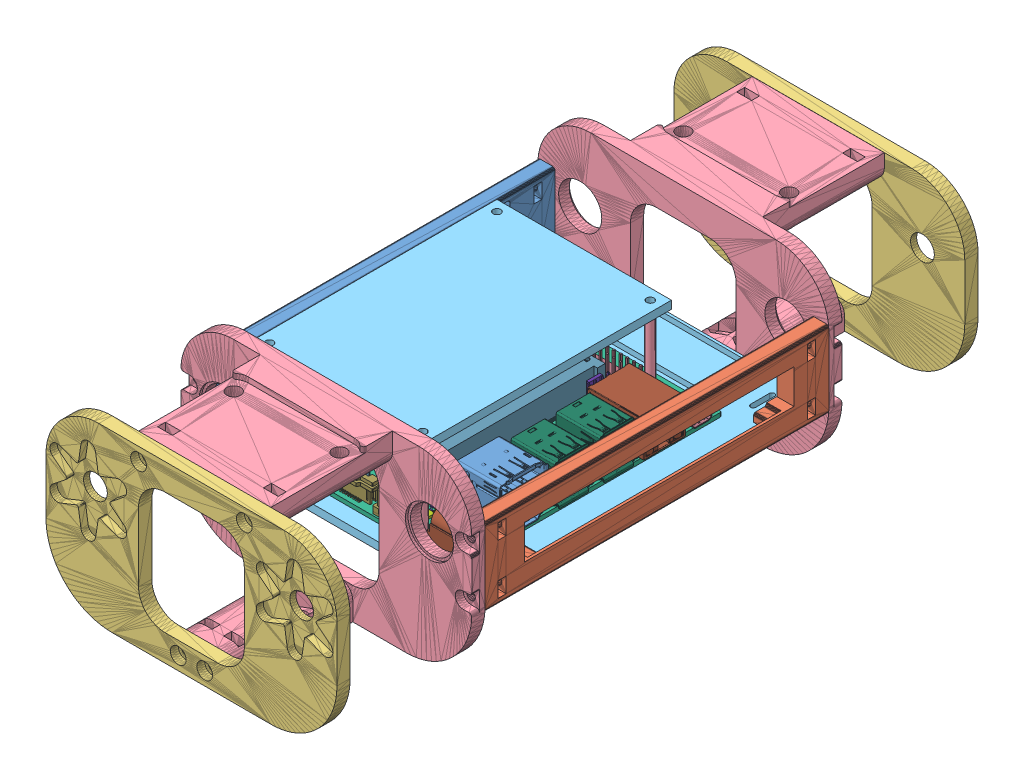
SolidWorks assembly torsol_with_jestson, configuration Default. Lengths in mm.
Overall size (110.41 70.14 242.41).
415 component instances, 78 part files, 32 mates.
Components (placement in the parent):
- R_side_plate-1: R_side_plate [Default] at (-145.3547 -0.5404 -42.0354) x (1 0 0) z (0 -1 0) size (6.5 130 29)
- non-mega_L_side_plate_jetson-2: non-mega_L_side_plate_jetson [Default] at (-41.8547 39.5958 -42.0354) x (-1 0 0) z (0 1 0) size (6.5 130 29)
- O_shoulder-1: O_shoulder [Default] at (-38.1905 81.6503 -93.0354) x (-1 0 0) z (0 -1 0) size (110 5.21 66)
- I_shoulder_mg-1: I_shoulder_mg [Default] at (-38.6047 81.5958 -42.0354) x (-1 0 0) z (0 -1 0) size (110 51 70)
- I_shoulder_mg-2: I_shoulder_mg [Default] at (-148.6047 81.4596 87.9646) x (1 0 0) z (0 -1 0) size (110 51 70)
- O_shoulder-2: O_shoulder [Default] at (-148.6047 81.4596 138.9646) x (1 0 0) z (0 -1 0) size (110 5.21 66)
- plate_with_jetson-1: plate_with_jetson [Default] at (-139.2728 38.0458 18.6623) x (-1 0 0) z (0 -1 0) size (107 134 44.9)
  - plate_jetson-1: plate_jetson [Default] at (-46.1681 -3.8023 -1.45) size (107 130 2.9)
  - Jetson nano_fixed.step-1: Jetson nano_fixed.step [Default] at (-69.1681 -61.3023 -1.45) x (0 1 0) z (0 0 -1) size (100 81.03 30.51)
    - 142-13449-1000-A02_ASM.step-1: 142-13449-1000-A02_ASM.step [Default] at origin size (100 81.03 23.19)
      - 142-13449-1000-A02.step-1: 142-13449-1000-A02.step [Default] at origin size (100 79 1.57)
      - 315-1109-000_1.step-1: 315-1109-000_1.step [Default] at (5.6 4.9 1.575) x (-1 0 0) z (0 0 1) size (4.5 3.5 0.8)
      - 0402_H040.step-1: 0402_H040.step [Default] at (8 -0.825 1.575) size (1 0.5 0.4)
      - 0402_H060.step-1: 0402_H060.step [Default] at (1 5 1.575) x (0 -1 0) z (0 0 1) size (1 0.5 0.6)
      - 0402_H040.step-2: 0402_H040.step [Default] at (9.9 -0.3 1.575) size (1 0.5 0.4)
      - 0402_H040.step-3: 0402_H040.step [Default] at (8.296 51.194 1.575) x (-1 0 0) z (0 0 1) size (1 0.5 0.4)
      - 0402_H040.step-4: 0402_H040.step [Default] at (76.2 36.9 1.575) x (-1 0 0) z (0 0 1) size (1 0.5 0.4)
      - 0402_H040.step-5: 0402_H040.step [Default] at (37.8 2.87 1.575) x (0 -1 0) z (0 0 1) size (1 0.5 0.4)
      - 0402_H040.step-6: 0402_H040.step [Default] at (38.6 2.87 1.575) x (0 -1 0) z (0 0 1) size (1 0.5 0.4)
      - 0402_H060.step-2: 0402_H060.step [Default] at (14.2 7.7 1.575) x (0 -1 0) z (0 0 1) size (1 0.5 0.6)
      - 0402_H040.step-7: 0402_H040.step [Default] at (64 27.5 1.575) x (-1 0 0) z (0 0 1) size (1 0.5 0.4)
      - 0402_H060.step-3: 0402_H060.step [Default] at (18.6 43.15 1.575) x (-1 0 0) z (0 0 1) size (1 0.5 0.6)
      - 0402_H060.step-4: 0402_H060.step [Default] at (65.5 52.8 1.575) x (0 1 0) z (0 0 1) size (1 0.5 0.6)
      - 0402_H060.step-5: 0402_H060.step [Default] at (64 28.4 1.575) x (-1 0 0) z (0 0 1) size (1 0.5 0.6)
      - 0402_H040.step-8: 0402_H040.step [Default] at (60.95 25.85 1.575) size (1 0.5 0.4)
      - 0402_H060.step-6: 0402_H060.step [Default] at (17.3 7.7 1.575) x (0 -1 0) z (0 0 1) size (1 0.5 0.6)
      - 0402_H060.step-7: 0402_H060.step [Default] at (18.6 7.7 1.575) x (0 -1 0) z (0 0 1) size (1 0.5 0.6)
      - 0402_H060.step-8: 0402_H060.step [Default] at (12.9 7.7 1.575) x (0 -1 0) z (0 0 1) size (1 0.5 0.6)
      - 0402_H060.step-9: 0402_H060.step [Default] at (80.9 37.7 1.575) x (-1 0 0) z (0 0 1) size (1 0.5 0.6)
      - 0402_H040.step-9: 0402_H040.step [Default] at (79.5 31.3 1.575) size (1 0.5 0.4)
      - 0402_H040.step-10: 0402_H040.step [Default] at (81 31.3 1.575) x (-1 0 0) z (0 0 1) size (1 0.5 0.4)
      - 0402_H060.step-10: 0402_H060.step [Default] at (79.3 37.7 1.575) size (1 0.5 0.6)
      - 0402_H060.step-11: 0402_H060.step [Default] at (74.8 4.05 1.575) x (-1 0 0) z (0 0 1) size (1 0.5 0.6)
      - 0402_H040.step-11: 0402_H040.step [Default] at (65.675 6.15 1.575) x (0 -1 0) z (0 0 1) size (1 0.5 0.4)
      - 0402_H060.step-12: 0402_H060.step [Default] at (67.7 6.85 1.575) x (0 1 0) z (0 0 1) size (1 0.5 0.6)
      - 0402_H040.step-12: 0402_H040.step [Default] at (64.475 5.8 1.575) x (-1 0 0) z (0 0 1) size (1 0.5 0.4)
      - 0402_H040.step-13: 0402_H040.step [Default] at (67.725 5.325 1.575) x (0 1 0) z (0 0 1) size (1 0.5 0.4)
      - 0402_H060.step-13: 0402_H060.step [Default] at (46.1 59.45 1.575) size (1 0.5 0.6)
      - 0402_H040.step-14: 0402_H040.step [Default] at (44.65 59.45 1.575) size (1 0.5 0.4)
      - 0402_H040.step-15: 0402_H040.step [Default] at (46.1 60.25 1.575) size (1 0.5 0.4)
      - 0402_H060.step-14: 0402_H060.step [Default] at (53.35 57.7 1.575) x (0 -1 0) z (0 0 1) size (1 0.5 0.6)
      - 0402_H040.step-16: 0402_H040.step [Default] at (47.6 59.45 1.575) size (1 0.5 0.4)
      - 0402_H040.step-17: 0402_H040.step [Default] at (48.4 60.25 1.575) size (1 0.5 0.4)
      - 0402_H040.step-18: 0402_H040.step [Default] at (47.7 58.325 1.575) x (0 1 0) z (0 0 1) size (1 0.5 0.4)
      - 0402_H060.step-15: 0402_H060.step [Default] at (46.5 58.65 1.575) x (-1 0 0) z (0 0 1) size (1 0.5 0.6)
      - 0402_H060.step-16: 0402_H060.step [Default] at (51.8 60.25 1.575) size (1 0.5 0.6)
      - 0402_H040.step-19: 0402_H040.step [Default] at (53.35 59.4 1.575) x (0 -1 0) z (0 0 1) size (1 0.5 0.4)
      - 0402_H040.step-20: 0402_H040.step [Default] at (50.2 60.25 1.575) x (-1 0 0) z (0 0 1) size (1 0.5 0.4)
      - 0402_H060.step-17: 0402_H060.step [Default] at (18.6 43.95 1.575) x (-1 0 0) z (0 0 1) size (1 0.5 0.6)
      - 0402_H060.step-18: 0402_H060.step [Default] at (52.75 2.9 1.575) x (0 -1 0) z (0 0 1) size (1 0.5 0.6)
      - 0402_H060.step-19: 0402_H060.step [Default] at (22.35 47.4 1.575) x (-1 0 0) z (0 0 1) size (1 0.5 0.6)
      - 0402_H060.step-20: 0402_H060.step [Default] at (20.55 47.4 1.575) x (-1 0 0) z (0 0 1) size (1 0.5 0.6)
      - 0402_H060.step-21: 0402_H060.step [Default] at (21.95 34.55 1.575) x (0 -1 0) z (0 0 1) size (1 0.5 0.6)
      - 0402_H060.step-22: 0402_H060.step [Default] at (21.05 34.55 1.575) x (0 -1 0) z (0 0 1) size (1 0.5 0.6)
      - 0402_H060.step-23: 0402_H060.step [Default] at (53.55 2.9 1.575) x (0 -1 0) z (0 0 1) size (1 0.5 0.6)
      - 0402_H060.step-24: 0402_H060.step [Default] at (25.4 54 1.575) x (-1 0 0) z (0 0 1) size (1 0.5 0.6)
      - 0402_H060.step-25: 0402_H060.step [Default] at (24 34.58 1.575) x (0 -1 0) z (0 0 1) size (1 0.5 0.6)
      - 0402_H040.step-21: 0402_H040.step [Default] at (55.6 2.95 1.575) x (0 -1 0) z (0 0 1) size (1 0.5 0.4)
      - 0402_H040.step-22: 0402_H040.step [Default] at (20.13 34.53 1.575) x (0 1 0) z (0 0 1) size (1 0.5 0.4)
      - 0402_H060.step-26: 0402_H060.step [Default] at (18.4 35.15 1.575) x (0 1 0) z (0 0 1) size (1 0.5 0.6)
      - 0402_H060.step-27: 0402_H060.step [Default] at (18.4 36.75 1.575) x (0 1 0) z (0 0 1) size (1 0.5 0.6)
      - 0402_H040.step-23: 0402_H040.step [Default] at (39.6 2.87 1.575) x (0 -1 0) z (0 0 1) size (1 0.5 0.4)
      - 0402_H040.step-24: 0402_H040.step [Default] at (40.4 2.87 1.575) x (0 -1 0) z (0 0 1) size (1 0.5 0.4)
      - 0402_H040.step-25: 0402_H040.step [Default] at (60.95 2.95 1.575) x (0 -1 0) z (0 0 1) size (1 0.5 0.4)
      - 0402_H040.step-26: 0402_H040.step [Default] at (60.15 2.95 1.575) x (0 -1 0) z (0 0 1) size (1 0.5 0.4)
      - 0402_H040.step-27: 0402_H040.step [Default] at (54.8 2.95 1.575) x (0 -1 0) z (0 0 1) size (1 0.5 0.4)
      - 0402_H040.step-28: 0402_H040.step [Default] at (31.6 54 1.575) size (1 0.5 0.4)
      - 0402_H040.step-29: 0402_H040.step [Default] at (27.4 54 1.575) size (1 0.5 0.4)
      - 0402_H040.step-30: 0402_H040.step [Default] at (29.6 54 1.575) x (-1 0 0) z (0 0 1) size (1 0.5 0.4)
      - 0402_H040.step-31: 0402_H040.step [Default] at (63.775 -14.475 1.575) size (1 0.5 0.4)
      - 0402_H040.step-32: 0402_H040.step [Default] at (63.775 -15.275 1.575) size (1 0.5 0.4)
      - 0402_H040.step-33: 0402_H040.step [Default] at (8.025 41.475 1.575) x (-1 0 0) z (0 0 1) size (1 0.5 0.4)
      - 0402_H060.step-28: 0402_H060.step [Default] at (63.95 1.25 1.575) x (0 1 0) z (0 0 1) size (1 0.5 0.6)
      - 0402_H060.step-29: 0402_H060.step [Default] at (2.95 54.05 1.575) x (0 1 0) z (0 0 1) size (1 0.5 0.6)
      - 0402_H040.step-34: 0402_H040.step [Default] at (92.2 -3.45 1.575) x (-1 0 0) z (0 0 1) size (1 0.5 0.4)
      - 0402_H060.step-30: 0402_H060.step [Default] at (32.85 7.7 1.575) x (0 -1 0) z (0 0 1) size (1 0.5 0.6)
      - 0402_H060.step-31: 0402_H060.step [Default] at (27.25 7.7 1.575) x (0 -1 0) z (0 0 1) size (1 0.5 0.6)
      - 0402_H060.step-32: 0402_H060.step [Default] at (31.25 7.7 1.575) x (0 -1 0) z (0 0 1) size (1 0.5 0.6)
      - 0402_H060.step-33: 0402_H060.step [Default] at (28.85 7.7 1.575) x (0 -1 0) z (0 0 1) size (1 0.5 0.6)
      - 0402_H060.step-34: 0402_H060.step [Default] at (32.05 7.7 1.575) x (0 -1 0) z (0 0 1) size (1 0.5 0.6)
      - 0402_H060.step-35: 0402_H060.step [Default] at (28.05 7.7 1.575) x (0 -1 0) z (0 0 1) size (1 0.5 0.6)
      - 0402_H060.step-36: 0402_H060.step [Default] at (30.45 7.7 1.575) x (0 -1 0) z (0 0 1) size (1 0.5 0.6)
      - 0402_H060.step-37: 0402_H060.step [Default] at (29.65 7.7 1.575) x (0 -1 0) z (0 0 1) size (1 0.5 0.6)
      - 0402_H060.step-38: 0402_H060.step [Default] at (24.65 6.41 1.575) x (0 -1 0) z (0 0 1) size (1 0.5 0.6)
      - 0402_H060.step-39: 0402_H060.step [Default] at (25.85 6.41 1.575) x (0 -1 0) z (0 0 1) size (1 0.5 0.6)
      - 0402_H060.step-40: 0402_H060.step [Default] at (4.2 36.5 1.575) x (0 1 0) z (0 0 1) size (1 0.5 0.6)
      - 0402_H060.step-41: 0402_H060.step [Default] at (89.7 4.7 1.575) x (0 -1 0) z (0 0 1) size (1 0.5 0.6)
      - 0402_H060.step-42: 0402_H060.step [Default] at (82.5 3.8 1.575) x (0 -1 0) z (0 0 1) size (1 0.5 0.6)
      - 0402_H060.step-43: 0402_H060.step [Default] at (12.65 49.7 1.575) size (1 0.5 0.6)
      - 0402_H060.step-44: 0402_H060.step [Default] at (11.2 50.15 1.575) x (0 -1 0) z (0 0 1) size (1 0.5 0.6)
      - 0402_H060.step-45: 0402_H060.step [Default] at (26.5 34.55 1.575) x (0 -1 0) z (0 0 1) size (1 0.5 0.6)
      - 0402_H060.step-46: 0402_H060.step [Default] at (29.9 34.5 1.575) x (0 -1 0) z (0 0 1) size (1 0.5 0.6)
      - 0402_H060.step-47: 0402_H060.step [Default] at (31.7 40.15 1.575) x (0 1 0) z (0 0 1) size (1 0.5 0.6)
      - 0402_H060.step-48: 0402_H060.step [Default] at (31.15 42.5 1.575) x (0 1 0) z (0 0 1) size (1 0.5 0.6)
      - 0402_H060.step-49: 0402_H060.step [Default] at (19.2 47.05 1.575) x (0 1 0) z (0 0 1) size (1 0.5 0.6)
      - 0402_H060.step-50: 0402_H060.step [Default] at (17.95 42 1.575) x (0 -1 0) z (0 0 1) size (1 0.5 0.6)
      - 0402_H060.step-51: 0402_H060.step [Default] at (27.3 48.25 1.575) x (0 1 0) z (0 0 1) size (1 0.5 0.6)
      - 0402_H060.step-52: 0402_H060.step [Default] at (31.7 37.85 1.575) x (0 -1 0) z (0 0 1) size (1 0.5 0.6)
      - 0402_H060.step-53: 0402_H060.step [Default] at (29.6 48.35 1.575) x (0 1 0) z (0 0 1) size (1 0.5 0.6)
      - 0402_H060.step-54: 0402_H060.step [Default] at (18.8 38.75 1.575) x (-1 0 0) z (0 0 1) size (1 0.5 0.6)
      - 0402_H060.step-55: 0402_H060.step [Default] at (18.7 57.2 1.575) x (0 -1 0) z (0 0 1) size (1 0.5 0.6)
      - 0402_H060.step-56: 0402_H060.step [Default] at (34.1 2.9 1.575) x (0 -1 0) z (0 0 1) size (1 0.5 0.6)
      - 0402_H060.step-57: 0402_H060.step [Default] at (35.8 2.9 1.575) x (0 -1 0) z (0 0 1) size (1 0.5 0.6)
      - 0402_H060.step-58: 0402_H060.step [Default] at (34.9 2.9 1.575) x (0 -1 0) z (0 0 1) size (1 0.5 0.6)
      - 0402_H060.step-59: 0402_H060.step [Default] at (36.6 2.9 1.575) x (0 -1 0) z (0 0 1) size (1 0.5 0.6)
      - 0402_H060.step-60: 0402_H060.step [Default] at (11.325 44.725 1.575) size (1 0.5 0.6)
      - 0402_H060.step-61: 0402_H060.step [Default] at (50.95 2.9 1.575) x (0 -1 0) z (0 0 1) size (1 0.5 0.6)
      - 0402_H060.step-62: 0402_H060.step [Default] at (51.75 2.9 1.575) x (0 -1 0) z (0 0 1) size (1 0.5 0.6)
      - 0402_H060.step-63: 0402_H060.step [Default] at (11.55 39.7 1.575) size (1 0.5 0.6)
      - 0402_H060.step-64: 0402_H060.step [Default] at (9.5 -8.5 1.575) x (-1 0 0) z (0 0 1) size (1 0.5 0.6)
      - 0402_H060.step-65: 0402_H060.step [Default] at (61.35 38.05 1.575) x (0 -1 0) z (0 0 1) size (1 0.5 0.6)
      - 0402_H060.step-66: 0402_H060.step [Default] at (60.55 38.05 1.575) x (0 -1 0) z (0 0 1) size (1 0.5 0.6)
      - 0402_H060.step-67: 0402_H060.step [Default] at (29.3 25.65 1.575) x (0 -1 0) z (0 0 1) size (1 0.5 0.6)
      - 0402_H060.step-68: 0402_H060.step [Default] at (63.3 56.2 1.575) x (0 1 0) z (0 0 1) size (1 0.5 0.6)
      - 0402_H060.step-69: 0402_H060.step [Default] at (20.5 54.2 1.575) size (1 0.5 0.6)
      - 0402_H060.step-70: 0402_H060.step [Default] at (60.1 32.15 1.575) x (0 1 0) z (0 0 1) size (1 0.5 0.6)
      - 0402_H060.step-71: 0402_H060.step [Default] at (60.9 32.15 1.575) x (0 1 0) z (0 0 1) size (1 0.5 0.6)
      - 0402_H060.step-72: 0402_H060.step [Default] at (18.6 44.85 1.575) size (1 0.5 0.6)
      - 0402_H060.step-73: 0402_H060.step [Default] at (18.6 45.65 1.575) size (1 0.5 0.6)
      - 0402_H060.step-74: 0402_H060.step [Default] at (18.1 27.25 1.575) size (1 0.5 0.6)
      - 0402_H060.step-75: 0402_H060.step [Default] at (15.1 7.7 1.575) x (0 -1 0) z (0 0 1) size (1 0.5 0.6)
      - 0402_H060.step-76: 0402_H060.step [Default] at (16.4 7.7 1.575) x (0 -1 0) z (0 0 1) size (1 0.5 0.6)
      - 0402_H060.step-77: 0402_H060.step [Default] at (20.8 7.7 1.575) x (0 -1 0) z (0 0 1) size (1 0.5 0.6)
      - 0402_H060.step-78: 0402_H060.step [Default] at (19.5 7.7 1.575) x (0 -1 0) z (0 0 1) size (1 0.5 0.6)
      - 0402_H060.step-79: 0402_H060.step [Default] at (21.9 2.8 1.575) size (1 0.5 0.6)
      - 0402_H060.step-80: 0402_H060.step [Default] at (12.75 29 1.575) size (1 0.5 0.6)
      - 0402_H060.step-81: 0402_H060.step [Default] at (10.225 5.1 1.575) size (1 0.5 0.6)
      - 0402_H060.step-82: 0402_H060.step [Default] at (22.8 27.65 1.575) x (0 1 0) z (0 0 1) size (1 0.5 0.6)
      - 0402_H060.step-83: 0402_H060.step [Default] at (18.85 25.15 1.575) x (0 -1 0) z (0 0 1) size (1 0.5 0.6)
      - 0402_H060.step-84: 0402_H060.step [Default] at (17.95 40.1 1.575) x (0 1 0) z (0 0 1) size (1 0.5 0.6)
      - 0402_H040.step-35: 0402_H040.step [Default] at (20.8 6.2 1.575) x (0 1 0) z (0 0 1) size (1 0.5 0.4)
      - 0402_H040.step-36: 0402_H040.step [Default] at (76 22.7 1.575) size (1 0.5 0.4)
      - 0402_H040.step-37: 0402_H040.step [Default] at (23.7 26.85 1.575) x (0 1 0) z (0 0 1) size (1 0.5 0.4)
      - 0402_H040.step-38: 0402_H040.step [Default] at (18 25.15 1.575) x (0 1 0) z (0 0 1) size (1 0.5 0.4)
      - 0402_H040.step-39: 0402_H040.step [Default] at (17.3 28.25 1.575) x (-1 0 0) z (0 0 1) size (1 0.5 0.4)
      - 0402_H040.step-40: 0402_H040.step [Default] at (13.15 4.2 1.575) x (0 -1 0) z (0 0 1) size (1 0.5 0.4)
      - 0402_H040.step-41: 0402_H040.step [Default] at (17.2 30.15 1.575) x (0 -1 0) z (0 0 1) size (1 0.5 0.4)
      - 0402_H040.step-42: 0402_H040.step [Default] at (14.2 6.2 1.575) x (0 1 0) z (0 0 1) size (1 0.5 0.4)
      - 0402_H040.step-43: 0402_H040.step [Default] at (12.9 6.2 1.575) x (0 1 0) z (0 0 1) size (1 0.5 0.4)
      - 0402_H040.step-44: 0402_H040.step [Default] at (15.1 6.2 1.575) x (0 1 0) z (0 0 1) size (1 0.5 0.4)
      - 0402_H040.step-45: 0402_H040.step [Default] at (16.4 6.2 1.575) x (0 1 0) z (0 0 1) size (1 0.5 0.4)
      - 0402_H040.step-46: 0402_H040.step [Default] at (19.5 6.2 1.575) x (0 1 0) z (0 0 1) size (1 0.5 0.4)
      - 0402_H040.step-47: 0402_H040.step [Default] at (17.3 6.2 1.575) x (0 1 0) z (0 0 1) size (1 0.5 0.4)
      - 0402_H040.step-48: 0402_H040.step [Default] at (18.6 6.2 1.575) x (0 1 0) z (0 0 1) size (1 0.5 0.4)
      - 0402_H040.step-49: 0402_H040.step [Default] at (24.2 24.55 1.575) x (0 1 0) z (0 0 1) size (1 0.5 0.4)
      - 0402_H040.step-50: 0402_H040.step [Default] at (23.5 54.9 1.575) x (0 1 0) z (0 0 1) size (1 0.5 0.4)
      - 0402_H040.step-51: 0402_H040.step [Default] at (13.2 39.75 1.575) x (-1 0 0) z (0 0 1) size (1 0.5 0.4)
      - 0402_H040.step-52: 0402_H040.step [Default] at (80.7 47.4 1.575) x (-1 0 0) z (0 0 1) size (1 0.5 0.4)
      - 0402_H040.step-53: 0402_H040.step [Default] at (77.5 22.7 1.575) x (-1 0 0) z (0 0 1) size (1 0.5 0.4)
      - 0402_H040.step-54: 0402_H040.step [Default] at (9.25 -12.75 1.575) x (-1 0 0) z (0 0 1) size (1 0.5 0.4)
      - 0402_H040.step-55: 0402_H040.step [Default] at (9.25 -11.95 1.575) x (-1 0 0) z (0 0 1) size (1 0.5 0.4)
      - 0402_H040.step-56: 0402_H040.step [Default] at (64.475 6.7 1.575) size (1 0.5 0.4)
      - 0402_H040.step-57: 0402_H040.step [Default] at (29.3 24 1.575) x (0 1 0) z (0 0 1) size (1 0.5 0.4)
      - 0402_H040.step-58: 0402_H040.step [Default] at (64.2 32.5 1.575) x (0 1 0) z (0 0 1) size (1 0.5 0.4)
      - 0402_H040.step-59: 0402_H040.step [Default] at (64.15 47.45 1.575) x (0 -1 0) z (0 0 1) size (1 0.5 0.4)
      - 0402_H040.step-60: 0402_H040.step [Default] at (64.2 31 1.575) x (0 -1 0) z (0 0 1) size (1 0.5 0.4)
      - 0402_H040.step-61: 0402_H040.step [Default] at (76.2 36.1 1.575) x (-1 0 0) z (0 0 1) size (1 0.5 0.4)
      - 0402_H040.step-62: 0402_H040.step [Default] at (78.4 45.15 1.575) size (1 0.5 0.4)
      - 0402_H040.step-63: 0402_H040.step [Default] at (81.7 38.6 1.575) size (1 0.5 0.4)
      - 0402_H040.step-64: 0402_H040.step [Default] at (81.7 39.4 1.575) size (1 0.5 0.4)
      - 0402_H040.step-65: 0402_H040.step [Default] at (59.35 51.825 1.575) size (1 0.5 0.4)
      - 0402_H040.step-66: 0402_H040.step [Default] at (60.825 51.825 1.575) x (-1 0 0) z (0 0 1) size (1 0.5 0.4)
      - 0402_H040.step-67: 0402_H040.step [Default] at (89.7 9.5 1.575) x (0 1 0) z (0 0 1) size (1 0.5 0.4)
      - 0402_H040.step-68: 0402_H040.step [Default] at (89.7 6.7 1.575) x (0 1 0) z (0 0 1) size (1 0.5 0.4)
      - 0402_H040.step-69: 0402_H040.step [Default] at (3.9 34.2 1.575) x (0 -1 0) z (0 0 1) size (1 0.5 0.4)
      - 0402_H040.step-70: 0402_H040.step [Default] at (5.1 35 1.575) x (0 1 0) z (0 0 1) size (1 0.5 0.4)
      - 0402_H040.step-71: 0402_H040.step [Default] at (32.85 5.81 1.575) x (0 -1 0) z (0 0 1) size (1 0.5 0.4)
      - 0402_H040.step-72: 0402_H040.step [Default] at (32.05 5.81 1.575) x (0 -1 0) z (0 0 1) size (1 0.5 0.4)
      - 0402_H040.step-73: 0402_H040.step [Default] at (27.25 5.81 1.575) x (0 -1 0) z (0 0 1) size (1 0.5 0.4)
      - 0402_H040.step-74: 0402_H040.step [Default] at (28.05 5.81 1.575) x (0 -1 0) z (0 0 1) size (1 0.5 0.4)
      - 0402_H040.step-75: 0402_H040.step [Default] at (31.25 5.81 1.575) x (0 -1 0) z (0 0 1) size (1 0.5 0.4)
      - 0402_H040.step-76: 0402_H040.step [Default] at (30.45 5.81 1.575) x (0 -1 0) z (0 0 1) size (1 0.5 0.4)
      - 0402_H040.step-77: 0402_H040.step [Default] at (28.85 5.81 1.575) x (0 -1 0) z (0 0 1) size (1 0.5 0.4)
      - 0402_H040.step-78: 0402_H040.step [Default] at (29.65 5.81 1.575) x (0 -1 0) z (0 0 1) size (1 0.5 0.4)
      - 0402_H040.step-79: 0402_H040.step [Default] at (13.5 52.9 1.575) x (-1 0 0) z (0 0 1) size (1 0.5 0.4)
      - 0402_H040.step-80: 0402_H040.step [Default] at (22.35 4 1.575) x (0 -1 0) z (0 0 1) size (1 0.5 0.4)
      - 0402_H040.step-81: 0402_H040.step [Default] at (21.55 4 1.575) x (0 1 0) z (0 0 1) size (1 0.5 0.4)
      - 0402_H040.step-82: 0402_H040.step [Default] at (25.85 4.9 1.575) x (0 -1 0) z (0 0 1) size (1 0.5 0.4)
      - 0402_H040.step-83: 0402_H040.step [Default] at (11.8 52.9 1.575) size (1 0.5 0.4)
      - 0402_H040.step-84: 0402_H040.step [Default] at (9.432 51.594 1.575) x (0 -1 0) z (0 0 1) size (1 0.5 0.4)
      - 0402_H040.step-85: 0402_H040.step [Default] at (8.975 50.3 1.575) size (1 0.5 0.4)
      - 0402_H040.step-86: 0402_H040.step [Default] at (82.8 -5.3 1.575) x (-1 0 0) z (0 0 1) size (1 0.5 0.4)
      - 0402_H040.step-87: 0402_H040.step [Default] at (82.4 -11.6 1.575) x (-1 0 0) z (0 0 1) size (1 0.5 0.4)
      - 0402_H040.step-88: 0402_H040.step [Default] at (22.8 26.05 1.575) x (0 1 0) z (0 0 1) size (1 0.5 0.4)
      - 0402_H040.step-89: 0402_H040.step [Default] at (20.8 28.25 1.575) size (1 0.5 0.4)
      - 0402_H040.step-90: 0402_H040.step [Default] at (20.8 24.65 1.575) x (-1 0 0) z (0 0 1) size (1 0.5 0.4)
      - 0402_H040.step-91: 0402_H040.step [Default] at (18.1 26.45 1.575) size (1 0.5 0.4)
      - 0402_H040.step-92: 0402_H040.step [Default] at (24.65 8.41 1.575) x (0 1 0) z (0 0 1) size (1 0.5 0.4)
      - 0402_H040.step-93: 0402_H040.step [Default] at (25.85 8.41 1.575) x (0 1 0) z (0 0 1) size (1 0.5 0.4)
      - 0402_H040.step-94: 0402_H040.step [Default] at (3.8 54.4 1.575) x (0 -1 0) z (0 0 1) size (1 0.5 0.4)
      - 0402_H040.step-95: 0402_H040.step [Default] at (2.45 44.45 1.575) x (0 -1 0) z (0 0 1) size (1 0.5 0.4)
      - 0402_H040.step-96: 0402_H040.step [Default] at (24.65 4.9 1.575) x (0 1 0) z (0 0 1) size (1 0.5 0.4)
      - 0402_H040.step-97: 0402_H040.step [Default] at (22.15 7.6 1.575) x (-1 0 0) z (0 0 1) size (1 0.5 0.4)
      - 0402_H040.step-98: 0402_H040.step [Default] at (79.2 47.4 1.575) size (1 0.5 0.4)
      - 0402_H040.step-99: 0402_H040.step [Default] at (19 28.25 1.575) size (1 0.5 0.4)
      - 0402_H040.step-100: 0402_H040.step [Default] at (9.65 9.7 1.575) x (0 -1 0) z (0 0 1) size (1 0.5 0.4)
      - 0402_H040.step-101: 0402_H040.step [Default] at (28.35 34.45 1.575) x (0 1 0) z (0 0 1) size (1 0.5 0.4)
      - 0402_H040.step-102: 0402_H040.step [Default] at (25.2 34.55 1.575) x (0 1 0) z (0 0 1) size (1 0.5 0.4)
      - 0402_H040.step-103: 0402_H040.step [Default] at (10.625 6.35 1.575) x (0 -1 0) z (0 0 1) size (1 0.5 0.4)
      - 0402_H040.step-104: 0402_H040.step [Default] at (9.825 6.35 1.575) x (0 1 0) z (0 0 1) size (1 0.5 0.4)
      - 0402_H040.step-105: 0402_H040.step [Default] at (4.775 42.975 1.575) x (0 1 0) z (0 0 1) size (1 0.5 0.4)
      - 0402_H040.step-106: 0402_H040.step [Default] at (19.8 32.9 1.575) x (-1 0 0) z (0 0 1) size (1 0.5 0.4)
      - 0402_H040.step-107: 0402_H040.step [Default] at (22.35 24.65 1.575) x (-1 0 0) z (0 0 1) size (1 0.5 0.4)
      - 0402_H040.step-108: 0402_H040.step [Default] at (62.4 54.7 1.575) size (1 0.5 0.4)
      - 0402_H040.step-109: 0402_H040.step [Default] at (62.2 60.05 1.575) x (-1 0 0) z (0 0 1) size (1 0.5 0.4)
      - 0402_H040.step-110: 0402_H040.step [Default] at (23.5 57.5 1.575) x (0 1 0) z (0 0 1) size (1 0.5 0.4)
      - 0402_H040.step-111: 0402_H040.step [Default] at (12.8 44.725 1.575) size (1 0.5 0.4)
      - 0402_H040.step-112: 0402_H040.step [Default] at (21.8 31.45 1.575) x (0 1 0) z (0 0 1) size (1 0.5 0.4)
      - 0402_H040.step-113: 0402_H040.step [Default] at (19.25 34.55 1.575) x (0 1 0) z (0 0 1) size (1 0.5 0.4)
      - 0402_H040.step-114: 0402_H040.step [Default] at (0.95 41.55 1.575) size (1 0.5 0.4)
      - 0402_H040.step-115: 0402_H040.step [Default] at (64.1 58 1.575) x (0 1 0) z (0 0 1) size (1 0.5 0.4)
      - 0402_H040.step-116: 0402_H040.step [Default] at (63.3 58 1.575) x (0 -1 0) z (0 0 1) size (1 0.5 0.4)
      - 0402_H040.step-117: 0402_H040.step [Default] at (63.55 59.7 1.575) x (0 -1 0) z (0 0 1) size (1 0.5 0.4)
      - 0402_H060.step-85: 0402_H060.step [Default] at (71.175 4 1.575) x (-1 0 0) z (0 0 1) size (1 0.5 0.6)
      - 0402_H040.step-118: 0402_H040.step [Default] at (86.6 -5.6 1.575) x (0 1 0) z (0 0 1) size (1 0.5 0.4)
      - 0402_H040.step-119: 0402_H040.step [Default] at (85.8 -5.3 1.575) x (0 1 0) z (0 0 1) size (1 0.5 0.4)
      - 0402_H040.step-120: 0402_H040.step [Default] at (10.25 51.6 1.575) x (0 1 0) z (0 0 1) size (1 0.5 0.4)
      - 0402_H040.step-121: 0402_H040.step [Default] at (80.5 28.55 1.575) size (1 0.5 0.4)
      - 0402_H040.step-122: 0402_H040.step [Default] at (13.95 4.2 1.575) x (0 -1 0) z (0 0 1) size (1 0.5 0.4)
      - 0402_H040.step-123: 0402_H040.step [Default] at (15.35 4.2 1.575) x (0 -1 0) z (0 0 1) size (1 0.5 0.4)
      - 0402_H040.step-124: 0402_H040.step [Default] at (16.15 4.2 1.575) x (0 -1 0) z (0 0 1) size (1 0.5 0.4)
      - 0402_H040.step-125: 0402_H040.step [Default] at (20.55 4.2 1.575) x (0 -1 0) z (0 0 1) size (1 0.5 0.4)
      - 0402_H040.step-126: 0402_H040.step [Default] at (19.75 4.2 1.575) x (0 -1 0) z (0 0 1) size (1 0.5 0.4)
      - 0402_H040.step-127: 0402_H040.step [Default] at (17.6 4.2 1.575) x (0 -1 0) z (0 0 1) size (1 0.5 0.4)
      - 0402_H040.step-128: 0402_H040.step [Default] at (18.4 4.2 1.575) x (0 -1 0) z (0 0 1) size (1 0.5 0.4)
      - 0402_H060.step-86: 0402_H060.step [Default] at (64.25 -13.325 1.575) x (0 -1 0) z (0 0 1) size (1 0.5 0.6)
      - 0402_H060.step-87: 0402_H060.step [Default] at (64.225 -11.825 1.575) x (0 1 0) z (0 0 1) size (1 0.5 0.6)
      - 0402_H040.step-129: 0402_H040.step [Default] at (63.8 -6.85 1.575) x (0 1 0) z (0 0 1) size (1 0.5 0.4)
      - 0402_H040.step-130: 0402_H040.step [Default] at (81.7 41.95 1.575) size (1 0.5 0.4)
      - 0402_H040.step-131: 0402_H040.step [Default] at (87.75 -6 1.575) x (-1 0 0) z (0 0 1) size (1 0.5 0.4)
      - 0402_H040.step-132: 0402_H040.step [Default] at (82.4 -13.6 1.575) x (-1 0 0) z (0 0 1) size (1 0.5 0.4)
      - 0402_H060.step-88: 0402_H060.step [Default] at (91.75 -5.95 1.575) size (1 0.5 0.6)
      - 0402_H040.step-133: 0402_H040.step [Default] at (3.65 49.25 1.575) x (0 -1 0) z (0 0 1) size (1 0.5 0.4)
      - 0402_H040.step-134: 0402_H040.step [Default] at (2.45 49.25 1.575) x (0 1 0) z (0 0 1) size (1 0.5 0.4)
      - 0402_H040.step-135: 0402_H040.step [Default] at (90.75 -1.45 1.575) x (-1 0 0) z (0 0 1) size (1 0.5 0.4)
      - 0402_H040.step-136: 0402_H040.step [Default] at (8.45 39.55 1.575) x (0 -1 0) z (0 0 1) size (1 0.5 0.4)
      - 0402_H060.step-89: 0402_H060.step [Default] at (8.85 -5.25 1.575) x (-1 0 0) z (0 0 1) size (1 0.5 0.6)
      - 0402_H040.step-137: 0402_H040.step [Default] at (18.6 32.55 1.575) x (0 1 0) z (0 0 1) size (1 0.5 0.4)
      - 0402_H060.step-90: 0402_H060.step [Default] at (4.5 44.45 1.575) x (0 1 0) z (0 0 1) size (1 0.5 0.6)
      - 0402_H040.step-138: 0402_H040.step [Default] at (8.35 2.75 1.575) size (1 0.5 0.4)
      - 0402_H040.step-139: 0402_H040.step [Default] at (9.4 1.95 1.575) size (1 0.5 0.4)
      - 0402_H040.step-140: 0402_H040.step [Default] at (8.2 1.55 1.575) x (0 1 0) z (0 0 1) size (1 0.5 0.4)
      - 0402_H060.step-91: 0402_H060.step [Default] at (8.5 3.875 1.575) x (0 -1 0) z (0 0 1) size (1 0.5 0.6)
      - 0402_H060.step-92: 0402_H060.step [Default] at (-0.8 41.5 1.575) x (-1 0 0) z (0 0 1) size (1 0.5 0.6)
      - 0402_H040.step-141: 0402_H040.step [Default] at (-1.35 7.75 1.575) size (1 0.5 0.4)
      - 0402_H040.step-142: 0402_H040.step [Default] at (8 0.425 1.575) size (1 0.5 0.4)
      - 0402_H040.step-143: 0402_H040.step [Default] at (67.9 4.025 1.575) x (-1 0 0) z (0 0 1) size (1 0.5 0.4)
      - 0402_H040.step-144: 0402_H040.step [Default] at (60.6 60.05 1.575) x (-1 0 0) z (0 0 1) size (1 0.5 0.4)
      - 0402_H040.step-145: 0402_H040.step [Default] at (72.85 4 1.575) x (-1 0 0) z (0 0 1) size (1 0.5 0.4)
      - 0402_H040.step-146: 0402_H040.step [Default] at (64.8 59.35 1.575) size (1 0.5 0.4)
      - 0402_H040.step-147: 0402_H040.step [Default] at (7.2 7.3 1.575) size (1 0.5 0.4)
      - 0402_H040.step-148: 0402_H040.step [Default] at (8.5 5.35 1.575) x (0 1 0) z (0 0 1) size (1 0.5 0.4)
      - 0402_H040.step-149: 0402_H040.step [Default] at (8.475 7.075 1.575) x (0 1 0) z (0 0 1) size (1 0.5 0.4)
      - VIRTUAL_SHORT.step-1: VIRTUAL_SHORT.step [Default] at (23.5 32.9 1.575) x (0 1 0) z (0 0 1) size (0.25 0.25 1)
      - VIRTUAL_SHORT.step-2: VIRTUAL_SHORT.step [Default] at (26.85 32.85 1.575) x (0 1 0) z (0 0 1) size (0.25 0.25 1)
      - VIRTUAL_SHORT.step-3: VIRTUAL_SHORT.step [Default] at (30.6 33.8 1.575) x (0 1 0) z (0 0 1) size (0.25 0.25 1)
      - VIRTUAL_SHORT.step-4: VIRTUAL_SHORT.step [Default] at (32.65 39.75 1.575) x (-1 0 0) z (0 0 1) size (0.25 0.25 1)
      - VIRTUAL_SHORT.step-5: VIRTUAL_SHORT.step [Default] at (31.85 42.1 1.575) x (-1 0 0) z (0 0 1) size (0.25 0.25 1)
      - VIRTUAL_SHORT.step-6: VIRTUAL_SHORT.step [Default] at (17.35 42.4 1.575) size (0.25 0.25 1)
      - VIRTUAL_SHORT.step-7: VIRTUAL_SHORT.step [Default] at (18.6 46.6 1.575) size (0.25 0.25 1)
      - VIRTUAL_SHORT.step-8: VIRTUAL_SHORT.step [Default] at (20.9 32.9 1.575) x (0 1 0) z (0 0 1) size (0.25 0.25 1)
      - VIRTUAL_SHORT.step-9: VIRTUAL_SHORT.step [Default] at (28.6 48.25 1.575) x (0 -1 0) z (0 0 1) size (0.25 0.25 1)
      - VIRTUAL_SHORT.step-10: VIRTUAL_SHORT.step [Default] at (27.1 49.35 1.575) x (0 -1 0) z (0 0 1) size (0.25 0.25 1)
      - VIRTUAL_SHORT.step-11: VIRTUAL_SHORT.step [Default] at (22.1 32.95 1.575) x (-1 0 0) z (0 0 1) size (0.25 0.25 1)
      - VIRTUAL_SHORT.step-12: VIRTUAL_SHORT.step [Default] at (32.65 38.25 1.575) x (-1 0 0) z (0 0 1) size (0.25 0.25 1)
      - VIRTUAL_SHORT.step-13: VIRTUAL_SHORT.step [Default] at (30.3 48 1.575) x (-1 0 0) z (0 0 1) size (0.25 0.25 1)
      - VIRTUAL_SHORT.step-14: VIRTUAL_SHORT.step [Default] at (17.15 38.95 1.575) size (0.25 0.25 1)
      - VIRTUAL_SHORT.step-15: VIRTUAL_SHORT.step [Default] at (17.15 39.7 1.575) size (0.25 0.25 1)
      - VIRTUAL_SHORT.step-16: VIRTUAL_SHORT.step [Default] at (76.175 4.1 1.575) x (-1 0 0) z (0 0 1) size (0.25 0.25 1)
      - 064-0377-000_2.step-1: 064-0377-000_2.step [Default] at (2 -4.75 1.575) x (0 -1 0) z (0 0 1) size (14.63 10.08 14.5)
      - 074-0117-000_2.step-1: 074-0117-000_2.step [Default] at (0.254 14.3 1.575) size (5.08 2.54 11.66)
      - 090-0096-000_1.step-1: 090-0096-000_1.step [Default] at (3.45 44.4 1.575) x (0 -1 0) z (0 0 1) size (1.2 0.6 0.4)
      - 090-0309-000_1.step-1: 090-0309-000_1.step [Default] at (-1.65 8.7 1.575) x (-1 0 0) z (0 0 1) size (1.2 0.6 0.4)
      - 115-1232-000_2.step-1: 115-1232-000_2.step [Default] at (1.25 6.5 1.575) x (-1 0 0) z (0 0 1) size (0.9 0.9 0.33)
